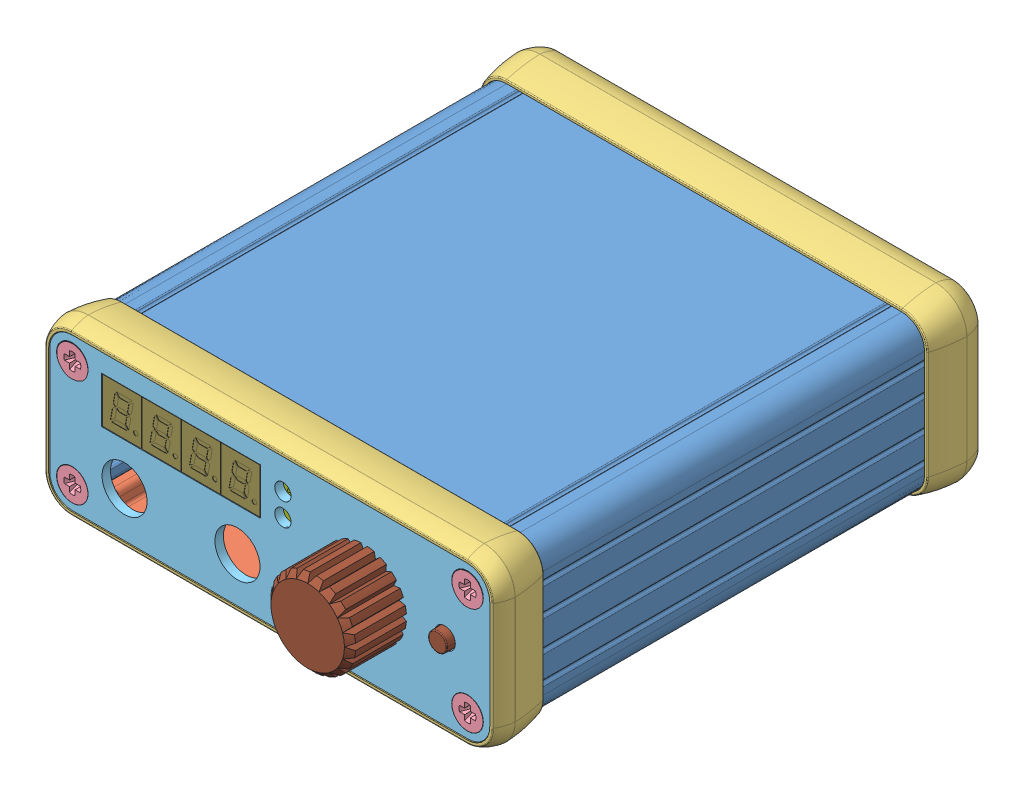
SolidWorks assembly Assembly_microbench_psu, configuration Standard. Lengths in mm. (continued)
Components (placement in the parent): (continued)
- main-board.step-1: main-board.step [Standard] at (-93.8915 -23.4474 -41.4) x (0 0 1) z (0 1 0) size (82.8 75 12.43) (continued)
  - IC305.step-1: IC305.step [Standard] at origin size (2.8 2.9 1.45) (continued)
    - 7556044960.step-1: 7556044960.step [Standard] at (41.9 44.6 0) size (2.8 2.91 1.45) (continued)
      - Leader-53.step-1: Leader-53.step [Standard] at (-0.8 -0.95 0) x (-1 0 0) z (0 0 1) size (0.6 0.51 0.78)
      - Leader-53.step-2: Leader-53.step [Standard] at (-0.8 0 0) x (-1 0 0) z (0 0 1) size (0.6 0.51 0.78)
      - Leader-53.step-3: Leader-53.step [Standard] at (-0.8 0.95 0) x (-1 0 0) z (0 0 1) size (0.6 0.51 0.78)
      - Leader-53.step-4: Leader-53.step [Standard] at (0.8 -0.95 0) size (0.6 0.51 0.78)
      - Leader-53.step-5: Leader-53.step [Standard] at (0.8 0.95 0) size (0.6 0.51 0.78)
  - IC304.step-1: IC304.step [Standard] at origin size (2.3 2 1.1)
    - 7556049760.step-1: 7556049760.step [Standard] at (41.5 41.6 0) size (2.3 2 1.1)
      - Body-11.step-1: Body-11.step [Standard] at (-0.625 -1 0) size (1.25 2 1.1)
        - Open CASCADE STEP translator 7.5 4.1.1-59.step-1: Open CASCADE STEP translator 7.5 4.1.1-59.step [Standard] at origin size (1.25 2 1.1)
      - Leader-60.step-1: Leader-60.step [Standard] at (-0.625 -0.65 0) x (-1 0 0) z (0 0 1) size (0.53 0.4 0.6)
      - Leader-60.step-2: Leader-60.step [Standard] at (-0.625 0 0) x (-1 0 0) z (0 0 1) size (0.53 0.4 0.6)
      - Leader-60.step-3: Leader-60.step [Standard] at (-0.625 0.65 0) x (-1 0 0) z (0 0 1) size (0.53 0.4 0.6)
      - Leader-60.step-4: Leader-60.step [Standard] at (0.625 -0.65 0) size (0.53 0.4 0.6)
      - Leader-60.step-5: Leader-60.step [Standard] at (0.625 0.65 0) size (0.53 0.4 0.6)
  - IC303.step-1: IC303.step [Standard] at origin size (4.1 4.1 0.8)
    - 7556056160.step-1: 7556056160.step [Standard] at (27.75 12.25 0) x (0 1 0) z (0 0 1) size (4.1 4.1 0.8)
      - Body-12.step-1: Body-12.step [Standard] at (-2.05 -2.05 0) size (4.1 4.1 0.8)
        - Open CASCADE STEP translator 7.5 3.2.1-61.step-1: Open CASCADE STEP translator 7.5 3.2.1-61.step [Standard] at origin size (4.1 4.1 0.8)
      - Pin Shape-3.step-1: Pin Shape-3.step [Standard] at (-2.05 -1.4 0) size (0.5 0.3 0.2)
        - Open CASCADE STEP translator 7.5 3.4.1.step-1: Open CASCADE STEP translator 7.5 3.4.1.step [Standard] at origin size (0.5 0.3 0.2)
      - Pin Shape-3.step-2: Pin Shape-3.step [Standard] at (-2.05 -0.9 0) size (0.5 0.3 0.2)
        - Open CASCADE STEP translator 7.5 3.4.1.step-1: Open CASCADE STEP translator 7.5 3.4.1.step [Standard] at origin size (0.5 0.3 0.2)
      - Pin Shape-3.step-3: Pin Shape-3.step [Standard] at (-2.05 -0.4 0) size (0.5 0.3 0.2)
        - Open CASCADE STEP translator 7.5 3.4.1.step-1: Open CASCADE STEP translator 7.5 3.4.1.step [Standard] at origin size (0.5 0.3 0.2)
      - Pin Shape-3.step-4: Pin Shape-3.step [Standard] at (-2.05 0.1 0) size (0.5 0.3 0.2)
        - Open CASCADE STEP translator 7.5 3.4.1.step-1: Open CASCADE STEP translator 7.5 3.4.1.step [Standard] at origin size (0.5 0.3 0.2)
      - Pin Shape-3.step-5: Pin Shape-3.step [Standard] at (-2.05 0.6 0) size (0.5 0.3 0.2)
        - Open CASCADE STEP translator 7.5 3.4.1.step-1: Open CASCADE STEP translator 7.5 3.4.1.step [Standard] at origin size (0.5 0.3 0.2)
      - Pin Shape-3.step-6: Pin Shape-3.step [Standard] at (-2.05 1.1 0) size (0.5 0.3 0.2)
        - Open CASCADE STEP translator 7.5 3.4.1.step-1: Open CASCADE STEP translator 7.5 3.4.1.step [Standard] at origin size (0.5 0.3 0.2)
      - Pin Shape-3.step-7: Pin Shape-3.step [Standard] at (2.05 -1.1 0) x (-1 0 0) z (0 0 1) size (0.5 0.3 0.2)
        - Open CASCADE STEP translator 7.5 3.4.1.step-1: Open CASCADE STEP translator 7.5 3.4.1.step [Standard] at origin size (0.5 0.3 0.2)
      - Pin Shape-3.step-8: Pin Shape-3.step [Standard] at (2.05 -0.6 0) x (-1 0 0) z (0 0 1) size (0.5 0.3 0.2)
        - Open CASCADE STEP translator 7.5 3.4.1.step-1: Open CASCADE STEP translator 7.5 3.4.1.step [Standard] at origin size (0.5 0.3 0.2)
      - Pin Shape-3.step-9: Pin Shape-3.step [Standard] at (2.05 -0.1 0) x (-1 0 0) z (0 0 1) size (0.5 0.3 0.2)
        - Open CASCADE STEP translator 7.5 3.4.1.step-1: Open CASCADE STEP translator 7.5 3.4.1.step [Standard] at origin size (0.5 0.3 0.2)
      - Pin Shape-3.step-10: Pin Shape-3.step [Standard] at (2.05 0.4 0) x (-1 0 0) z (0 0 1) size (0.5 0.3 0.2)
        - Open CASCADE STEP translator 7.5 3.4.1.step-1: Open CASCADE STEP translator 7.5 3.4.1.step [Standard] at origin size (0.5 0.3 0.2)
      - Pin Shape-3.step-11: Pin Shape-3.step [Standard] at (2.05 0.9 0) x (-1 0 0) z (0 0 1) size (0.5 0.3 0.2)
        - Open CASCADE STEP translator 7.5 3.4.1.step-1: Open CASCADE STEP translator 7.5 3.4.1.step [Standard] at origin size (0.5 0.3 0.2)
      - Pin Shape-3.step-12: Pin Shape-3.step [Standard] at (2.05 1.4 0) x (-1 0 0) z (0 0 1) size (0.5 0.3 0.2)
        - Open CASCADE STEP translator 7.5 3.4.1.step-1: Open CASCADE STEP translator 7.5 3.4.1.step [Standard] at origin size (0.5 0.3 0.2)
      - Open CASCADE STEP translator 7.5 3.1-62.step-1: Open CASCADE STEP translator 7.5 3.1-62.step [Standard] at (-2.05 -2.05 0) size (0.52 0.52 0.01)
      - Thermal Shape-63.step-1: Thermal Shape-63.step [Standard] at (-1.325 -1.69 -0.001) size (2.65 3.38 0)
  - IC302.step-1: IC302.step [Standard] at origin size (3.1 3.1 1)
    - 8362585520.step-1: 8362585520.step [Standard] at (43.633 32.962 0) size (3.1 3.1 1)
      - Extruded-64.step-1: Extruded-64.step [Standard] at origin size (3.1 3.1 1)
  - IC300.step-1: IC300.step [Standard] at origin size (4.1 4.1 0.8)
    - 7556056160.step-1: 7556056160.step [Standard] at (32.75 12.25 0) x (0 1 0) z (0 0 1) size (4.1 4.1 0.8)
      - Body-12.step-1: Body-12.step [Standard] at (-2.05 -2.05 0) size (4.1 4.1 0.8)
        - Open CASCADE STEP translator 7.5 3.2.1-61.step-1: Open CASCADE STEP translator 7.5 3.2.1-61.step [Standard] at origin size (4.1 4.1 0.8)
      - Pin Shape-3.step-1: Pin Shape-3.step [Standard] at (-2.05 -1.4 0) size (0.5 0.3 0.2)
        - Open CASCADE STEP translator 7.5 3.4.1.step-1: Open CASCADE STEP translator 7.5 3.4.1.step [Standard] at origin size (0.5 0.3 0.2)
      - Pin Shape-3.step-2: Pin Shape-3.step [Standard] at (-2.05 -0.9 0) size (0.5 0.3 0.2)
        - Open CASCADE STEP translator 7.5 3.4.1.step-1: Open CASCADE STEP translator 7.5 3.4.1.step [Standard] at origin size (0.5 0.3 0.2)
      - Pin Shape-3.step-3: Pin Shape-3.step [Standard] at (-2.05 -0.4 0) size (0.5 0.3 0.2)
        - Open CASCADE STEP translator 7.5 3.4.1.step-1: Open CASCADE STEP translator 7.5 3.4.1.step [Standard] at origin size (0.5 0.3 0.2)
      - Pin Shape-3.step-4: Pin Shape-3.step [Standard] at (-2.05 0.1 0) size (0.5 0.3 0.2)
        - Open CASCADE STEP translator 7.5 3.4.1.step-1: Open CASCADE STEP translator 7.5 3.4.1.step [Standard] at origin size (0.5 0.3 0.2)
      - Pin Shape-3.step-5: Pin Shape-3.step [Standard] at (-2.05 0.6 0) size (0.5 0.3 0.2)
        - Open CASCADE STEP translator 7.5 3.4.1.step-1: Open CASCADE STEP translator 7.5 3.4.1.step [Standard] at origin size (0.5 0.3 0.2)
      - Pin Shape-3.step-6: Pin Shape-3.step [Standard] at (-2.05 1.1 0) size (0.5 0.3 0.2)
        - Open CASCADE STEP translator 7.5 3.4.1.step-1: Open CASCADE STEP translator 7.5 3.4.1.step [Standard] at origin size (0.5 0.3 0.2)
      - Pin Shape-3.step-7: Pin Shape-3.step [Standard] at (2.05 -1.1 0) x (-1 0 0) z (0 0 1) size (0.5 0.3 0.2)
        - Open CASCADE STEP translator 7.5 3.4.1.step-1: Open CASCADE STEP translator 7.5 3.4.1.step [Standard] at origin size (0.5 0.3 0.2)
      - Pin Shape-3.step-8: Pin Shape-3.step [Standard] at (2.05 -0.6 0) x (-1 0 0) z (0 0 1) size (0.5 0.3 0.2)
        - Open CASCADE STEP translator 7.5 3.4.1.step-1: Open CASCADE STEP translator 7.5 3.4.1.step [Standard] at origin size (0.5 0.3 0.2)
      - Pin Shape-3.step-9: Pin Shape-3.step [Standard] at (2.05 -0.1 0) x (-1 0 0) z (0 0 1) size (0.5 0.3 0.2)
        - Open CASCADE STEP translator 7.5 3.4.1.step-1: Open CASCADE STEP translator 7.5 3.4.1.step [Standard] at origin size (0.5 0.3 0.2)
      - Pin Shape-3.step-10: Pin Shape-3.step [Standard] at (2.05 0.4 0) x (-1 0 0) z (0 0 1) size (0.5 0.3 0.2)
        - Open CASCADE STEP translator 7.5 3.4.1.step-1: Open CASCADE STEP translator 7.5 3.4.1.step [Standard] at origin size (0.5 0.3 0.2)
      - Pin Shape-3.step-11: Pin Shape-3.step [Standard] at (2.05 0.9 0) x (-1 0 0) z (0 0 1) size (0.5 0.3 0.2)
        - Open CASCADE STEP translator 7.5 3.4.1.step-1: Open CASCADE STEP translator 7.5 3.4.1.step [Standard] at origin size (0.5 0.3 0.2)
      - Pin Shape-3.step-12: Pin Shape-3.step [Standard] at (2.05 1.4 0) x (-1 0 0) z (0 0 1) size (0.5 0.3 0.2)
        - Open CASCADE STEP translator 7.5 3.4.1.step-1: Open CASCADE STEP translator 7.5 3.4.1.step [Standard] at origin size (0.5 0.3 0.2)
      - Open CASCADE STEP translator 7.5 3.1-62.step-1: Open CASCADE STEP translator 7.5 3.1-62.step [Standard] at (-2.05 -2.05 0) size (0.52 0.52 0.01)
      - Thermal Shape-63.step-1: Thermal Shape-63.step [Standard] at (-1.325 -1.69 -0.001) size (2.65 3.38 0)
  - C315.step-1: C315.step [Standard] at origin size (0.65 1.15 0.65)
    - 7876647632.step-1: 7876647632.step [Standard] at (45.9 43.8 0) x (0 -1 0) z (0 0 1) size (1.15 0.65 0.65)
      - Terminal-6.step-1: Terminal-6.step [Standard] at (-0.575 -0.325 0) size (1.15 0.65 0.65)
        - Open CASCADE STEP translator 6.8 5.1.1-9.step-1: Open CASCADE STEP translator 6.8 5.1.1-9.step [Standard] at origin size (0.15 0.65 0.65)
        - Open CASCADE STEP translator 6.8 5.1.2-10.step-1: Open CASCADE STEP translator 6.8 5.1.2-10.step [Standard] at origin size (0.15 0.65 0.65)
      - Mid_Body-3.step-1: Mid_Body-3.step [Standard] at (-0.575 -0.325 0) size (0.85 0.65 0.65)
        - Open CASCADE STEP translator 6.8 5.2.1-11.step-1: Open CASCADE STEP translator 6.8 5.2.1-11.step [Standard] at origin size (0.85 0.65 0.65)
  - C314.step-1: C314.step [Standard] at origin size (0.65 1.15 0.65)
    - 7876647632.step-1: 7876647632.step [Standard] at (44.9 41.9 0) x (0 -1 0) z (0 0 1) size (1.15 0.65 0.65)
      - Terminal-6.step-1: Terminal-6.step [Standard] at (-0.575 -0.325 0) size (1.15 0.65 0.65)
        - Open CASCADE STEP translator 6.8 5.1.1-9.step-1: Open CASCADE STEP translator 6.8 5.1.1-9.step [Standard] at origin size (0.15 0.65 0.65)
        - Open CASCADE STEP translator 6.8 5.1.2-10.step-1: Open CASCADE STEP translator 6.8 5.1.2-10.step [Standard] at origin size (0.15 0.65 0.65)
      - Mid_Body-3.step-1: Mid_Body-3.step [Standard] at (-0.575 -0.325 0) size (0.85 0.65 0.65)
        - Open CASCADE STEP translator 6.8 5.2.1-11.step-1: Open CASCADE STEP translator 6.8 5.2.1-11.step [Standard] at origin size (0.85 0.65 0.65)
  - C313.step-1: C313.step [Standard] at origin size (0.65 1.15 0.65)
    - 7876639952.step-1: 7876639952.step [Standard] at (45.9 45.7 0) x (0 1 0) z (0 0 1) size (1.15 0.65 0.65)
      - Terminal-3.step-1: Terminal-3.step [Standard] at (-0.575 -0.325 0) size (1.15 0.65 0.65)
        - Open CASCADE STEP translator 6.8 5.1.1-4.step-1: Open CASCADE STEP translator 6.8 5.1.1-4.step [Standard] at origin size (0.15 0.65 0.65)
        - Open CASCADE STEP translator 6.8 5.1.2-5.step-1: Open CASCADE STEP translator 6.8 5.1.2-5.step [Standard] at origin size (0.15 0.65 0.65)
      - Mid_Body-2.step-1: Mid_Body-2.step [Standard] at (-0.575 -0.325 0) size (0.85 0.65 0.65)
        - Open CASCADE STEP translator 6.8 5.2.1-6.step-1: Open CASCADE STEP translator 6.8 5.2.1-6.step [Standard] at origin size (0.85 0.65 0.65)
  - C312.step-1: C312.step [Standard] at origin size (0.65 1.15 0.65)
    - 7876639952.step-1: 7876639952.step [Standard] at (50.6 41.9 0) x (0 1 0) z (0 0 1) size (1.15 0.65 0.65)
      - Terminal-3.step-1: Terminal-3.step [Standard] at (-0.575 -0.325 0) size (1.15 0.65 0.65)
        - Open CASCADE STEP translator 6.8 5.1.1-4.step-1: Open CASCADE STEP translator 6.8 5.1.1-4.step [Standard] at origin size (0.15 0.65 0.65)
        - Open CASCADE STEP translator 6.8 5.1.2-5.step-1: Open CASCADE STEP translator 6.8 5.1.2-5.step [Standard] at origin size (0.15 0.65 0.65)
      - Mid_Body-2.step-1: Mid_Body-2.step [Standard] at (-0.575 -0.325 0) size (0.85 0.65 0.65)
        - Open CASCADE STEP translator 6.8 5.2.1-6.step-1: Open CASCADE STEP translator 6.8 5.2.1-6.step [Standard] at origin size (0.85 0.65 0.65)
  - C311.step-1: C311.step [Standard] at origin size (0.65 1.15 0.65)
    - 7876647632.step-1: 7876647632.step [Standard] at (39.2 43.7 0) x (0 -1 0) z (0 0 1) size (1.15 0.65 0.65)
      - Terminal-6.step-1: Terminal-6.step [Standard] at (-0.575 -0.325 0) size (1.15 0.65 0.65)
        - Open CASCADE STEP translator 6.8 5.1.1-9.step-1: Open CASCADE STEP translator 6.8 5.1.1-9.step [Standard] at origin size (0.15 0.65 0.65)
        - Open CASCADE STEP translator 6.8 5.1.2-10.step-1: Open CASCADE STEP translator 6.8 5.1.2-10.step [Standard] at origin size (0.15 0.65 0.65)
      - Mid_Body-3.step-1: Mid_Body-3.step [Standard] at (-0.575 -0.325 0) size (0.85 0.65 0.65)
        - Open CASCADE STEP translator 6.8 5.2.1-11.step-1: Open CASCADE STEP translator 6.8 5.2.1-11.step [Standard] at origin size (0.85 0.65 0.65)
  - C310.step-1: C310.step [Standard] at origin size (0.65 1.15 0.65)
    - 7876647632.step-1: 7876647632.step [Standard] at (38.1 41.3 0) x (0 -1 0) z (0 0 1) size (1.15 0.65 0.65)
      - Terminal-6.step-1: Terminal-6.step [Standard] at (-0.575 -0.325 0) size (1.15 0.65 0.65)
        - Open CASCADE STEP translator 6.8 5.1.1-9.step-1: Open CASCADE STEP translator 6.8 5.1.1-9.step [Standard] at origin size (0.15 0.65 0.65)
        - Open CASCADE STEP translator 6.8 5.1.2-10.step-1: Open CASCADE STEP translator 6.8 5.1.2-10.step [Standard] at origin size (0.15 0.65 0.65)
      - Mid_Body-3.step-1: Mid_Body-3.step [Standard] at (-0.575 -0.325 0) size (0.85 0.65 0.65)
        - Open CASCADE STEP translator 6.8 5.2.1-11.step-1: Open CASCADE STEP translator 6.8 5.2.1-11.step [Standard] at origin size (0.85 0.65 0.65)
  - C309.step-1: C309.step [Standard] at origin size (0.65 1.15 0.65)
    - 7876639952.step-1: 7876639952.step [Standard] at (39.2 45.6 0) x (0 1 0) z (0 0 1) size (1.15 0.65 0.65)
      - Terminal-3.step-1: Terminal-3.step [Standard] at (-0.575 -0.325 0) size (1.15 0.65 0.65)
        - Open CASCADE STEP translator 6.8 5.1.1-4.step-1: Open CASCADE STEP translator 6.8 5.1.1-4.step [Standard] at origin size (0.15 0.65 0.65)
        - Open CASCADE STEP translator 6.8 5.1.2-5.step-1: Open CASCADE STEP translator 6.8 5.1.2-5.step [Standard] at origin size (0.15 0.65 0.65)
      - Mid_Body-2.step-1: Mid_Body-2.step [Standard] at (-0.575 -0.325 0) size (0.85 0.65 0.65)
        - Open CASCADE STEP translator 6.8 5.2.1-6.step-1: Open CASCADE STEP translator 6.8 5.2.1-6.step [Standard] at origin size (0.85 0.65 0.65)
  - C308.step-1: C308.step [Standard] at origin size (0.65 1.15 0.65)
    - 7876639952.step-1: 7876639952.step [Standard] at (43.8 41.9 0) x (0 1 0) z (0 0 1) size (1.15 0.65 0.65)
      - Terminal-3.step-1: Terminal-3.step [Standard] at (-0.575 -0.325 0) size (1.15 0.65 0.65)
        - Open CASCADE STEP translator 6.8 5.1.1-4.step-1: Open CASCADE STEP translator 6.8 5.1.1-4.step [Standard] at origin size (0.15 0.65 0.65)
        - Open CASCADE STEP translator 6.8 5.1.2-5.step-1: Open CASCADE STEP translator 6.8 5.1.2-5.step [Standard] at origin size (0.15 0.65 0.65)
      - Mid_Body-2.step-1: Mid_Body-2.step [Standard] at (-0.575 -0.325 0) size (0.85 0.65 0.65)
        - Open CASCADE STEP translator 6.8 5.2.1-6.step-1: Open CASCADE STEP translator 6.8 5.2.1-6.step [Standard] at origin size (0.85 0.65 0.65)
- Knob-1: Knob [Standard] at (-39.3785 -22.2724 43.2) x (1 0 0) z (0 -1 0) size (14.96 10 14.96)
Mates (geometry in assembly coordinates):
- Distance1: distance = 0.1 mm anti-aligned: plane of Front Cover-1 through (-95.3565 -12.7454 42.9) normal (-1 0 0); plane of 1455J801BK.step-1/K Bezel.step-1 through (-95.4565 -31.8404 41.4) normal (1 0 0)
- Distance2: distance = 0.1 mm anti-aligned: plane of Front Cover-1 through (-21.3135 -8.8104 42.9) normal (0 1 0); plane of 1455J801BK.step-1/K Bezel.step-1 through (-91.4565 -8.7104 41.4) normal (0 -1 0)
- Coincident3: coincident anti-aligned: plane of 1455J801BK.step-1/K Bezel.step-1 through (-94.7065 -12.7104 41.4) normal (0 0 1); plane of Front Cover-1 through (-91.4215 -31.7994 41.4) normal (0 0 -1)
- Distance3: distance = 0.1 mm anti-aligned: plane of Back Cover-1 through (-21.3135 -8.8104 -41.4) normal (0 1 0); plane of 1455J801BK.step-1/K Bezel.step-2 through (-21.3265 -8.7104 -41.4) normal (0 -1 0)
- Distance4: distance = 0.1 mm anti-aligned: plane of 1455J801BK.step-1/K Bezel.step-2 through (-95.4565 -12.7104 -41.4) normal (1 0 0); plane of Back Cover-1 through (-95.3565 -12.7454 -41.4) normal (-1 0 0)
- Coincident6: coincident anti-aligned: plane of 1455J801BK.step-1/K Bezel.step-2 through (-94.7065 -31.8404 -41.4) normal (0 0 -1); plane of Back Cover-1 through (-91.4215 -31.7994 -41.4) normal (0 0 1)
- Concentric1: concentric aligned: circle of Front Cover-1; cylinder of display-board.step-1/Board.step-1/Open CASCADE STEP translator 7.5 4.1.1.step-1 through (-49.1175 -13.0604 38.3798) axis (0 0 -1) radius 1.05
- Concentric2: concentric aligned: cylinder of Front Cover-1 through (-87.8675 -19.2604 39.8) axis (0 0 1) radius 0.9; circle of display-board.step-1/Board.step-1/Open CASCADE STEP translator 7.5 4.1.1.step-1
- Coincident7: coincident anti-aligned: plane of Front Cover-1 through (-49.1175 -13.0604 39.8) normal (0 0 -1); plane of display-board.step-1/Board.step-1/Open CASCADE STEP translator 7.5 4.1.1.step-1 through (-68.4925 -16.1604 39.8) normal (0 0 1)
- Concentric3: concentric anti-aligned: circle of Front Cover-1; circle of ui-board.step-1/Board.step-1/Open CASCADE STEP translator 7.5 2.1.1.step-1
- Concentric4: concentric aligned: cylinder of Front Cover-1 through (-49.6285 -29.7724 36.6) axis (0 0 1) radius 0.9; circle of ui-board.step-1/Board.step-1/Open CASCADE STEP translator 7.5 2.1.1.step-1
- Coincident8: coincident anti-aligned: plane of Front Cover-1 through (-28.1285 -14.7724 36.6) normal (0 0 -1); plane of ui-board.step-1/Board.step-1/Open CASCADE STEP translator 7.5 2.1.1.step-1 through (-36.2363 -22.6646 36.6) normal (0 0 1)
- Distance5: distance = 0.1 mm: plane of main-board.step-1/Board.step-1/Open CASCADE STEP translator 7.5 3.1.1.step-1 through (-57.364 -24.8676 2.653) normal (0 -1 0); plane of 1455J801BK.step-1/J Channel Extrusion 80mm.step-1 through (-18.8915 -24.9676 0) normal (0 1 0)
- Coincident10: coincident: plane of 1455J801BK.step-1/J Channel Extrusion 80mm.step-1 through (-18.8915 -22.9676 0) normal (-1 0 0); plane of main-board.step-1/Board.step-1/Open CASCADE STEP translator 7.5 3.1.1.step-1 through (-18.8915 -24.8676 41.4) normal (1 0 0)
- Coincident11: coincident anti-aligned: plane of Front Cover-1 through (-91.4215 -31.7994 41.4) normal (0 0 -1); plane of main-board.step-1/Board.step-1/Open CASCADE STEP translator 7.5 3.1.1.step-1 through (-54.8915 -24.8676 41.4) normal (0 0 1)
- Concentric5: concentric: cylinder of ui-board.step-1/SW1.step-1/PEC11S-929K-S0015_RGB8421504.step-1 through (-39.3785 -22.2724 41.2127) axis (0 0 1) radius 3.5; cylinder of Knob-1 through (-39.3785 -22.2724 43.2) axis (0 0 -1) radius 4
- Distance6: distance = 0.3 mm anti-aligned: plane of Knob-1 through (-31.8785 -22.2724 43.2) normal (0 0 -1); plane of Front Cover-1 through (-91.4215 -31.7994 42.9) normal (0 0 1)
